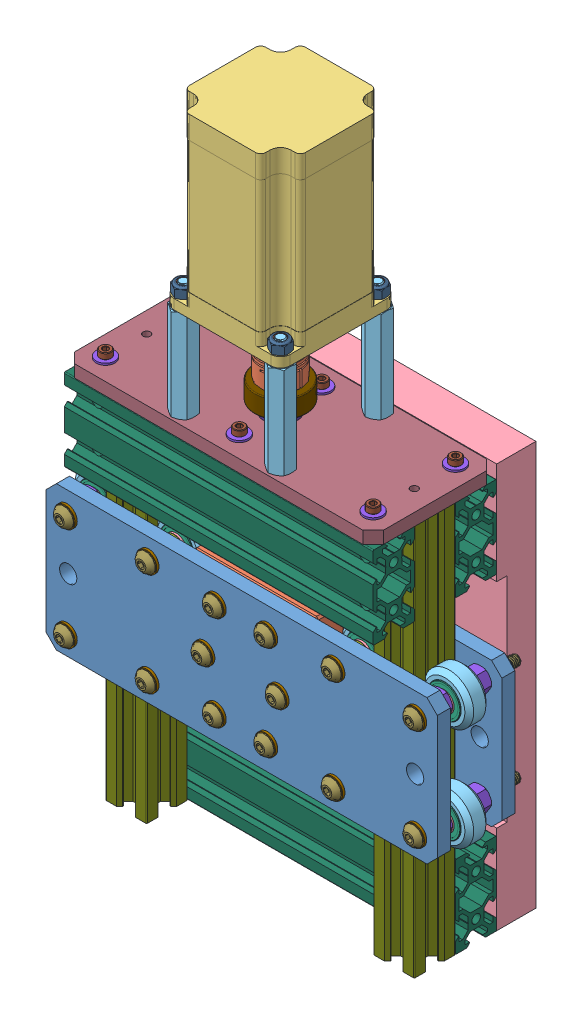
SolidWorks assembly Longitudinal Trim Assembly, configuration Default. Lengths in mm.
Overall size (193.6 327 79.96).
284 component instances, 29 part files, 72 mates.
Components (placement in the parent):
- Trim Sled Assembly-1: Trim Sled Assembly [Default] at origin size (193.6 74.69 53.02)
  - Trim Sled Plate-1: Trim Sled Plate [Default] at origin size (190 70 6.35)
  - Lead Screw Nut Clamshell-1: Lead Screw Nut Clamshell [Default] at origin size (60 70 12.5)
  - MISUMI Brass Lead Screw Flange Nut - MTSGR12-1: MISUMI Brass Lead Screw Flange Nut - MTSGR12 [Default] at (0 -15 30) x (0 1 0) z (0 0 1) size (30 44 24)
  - Lead Screw Nut Clamshell-2: Lead Screw Nut Clamshell [Default] at (0 0 60) x (-1 0 0) z (0 0 -1) size (60 70 12.5)
  - Inboard Wheel Stack-1: Inboard Wheel Stack [Default] at (-45.15 -25 23.5) size (23.9 23.9 25)
    - Xtreme Solid V Wheel Kit Assembly-1: Xtreme Solid V Wheel Kit Assembly [Default] at origin size (23.9 23.9 13)
      - Precision Shim - 10x5x1mm-1: Precision Shim - 10x5x1mm [Default] at origin size (10 10 1)
      - Xtreme Solid V Wheel Assembly-1: Xtreme Solid V Wheel Assembly [Default] at (45.15 25 -23.5) size (23.9 23.9 11)
        - Xtreme Solid V Wheel-1: Xtreme Solid V Wheel [Default] at (-45.15 -25 30) x (0 0 1) z (-1 0 0) size (10.2 23.9 23.9)
        - Wheel+Kit+-+5x16x5mm+Sealed+Radial+Ball+Bearing.step.f3d-1: Wheel+Kit+-+5x16x5mm+Sealed+Radial+Ball+Bearing.step.f3d [Default] at (-45.15 -25 30) x (0 1 0) z (-1 0 0) size (16 5 16)
        - Wheel+Kit+-+5x16x5mm+Sealed+Radial+Ball+Bearing.step.f3d-2: Wheel+Kit+-+5x16x5mm+Sealed+Radial+Ball+Bearing.step.f3d [Default] at (-45.15 -25 30) x (0 1 0) z (1 0 0) size (16 5 16)
      - Precision Shim - 10x5x1mm-2: Precision Shim - 10x5x1mm [Default] at (0 0 12) size (10 10 1)
    - Aluminum Spacer 6mm-1: Aluminum Spacer 6mm [Default] at (0 0 -6) size (10 10 6)
    - Aluminum Spacer 6mm-2: Aluminum Spacer 6mm [Default] at (0 0 13) size (10 10 6)
  - Inboard Wheel Stack_1-1: Inboard Wheel Stack_1 [Default] at (-45.15 25 23.5) size (23.9 23.9 25)
    - Xtreme Solid V Wheel Kit Assembly_1-1: Xtreme Solid V Wheel Kit Assembly_1 [Default] at origin size (23.9 23.9 13)
      - Precision Shim - 10x5x1mm-1: Precision Shim - 10x5x1mm [Default] at origin size (10 10 1)
      - Xtreme Solid V Wheel Assembly_1-1: Xtreme Solid V Wheel Assembly_1 [Default] at (45.15 55 -23.5) size (23.9 23.9 11)
        - Xtreme Solid V Wheel-1: Xtreme Solid V Wheel [Default] at (-45.15 -55 30) x (0 0 1) z (-1 0 0) size (10.2 23.9 23.9)
        - Wheel+Kit+-+5x16x5mm+Sealed+Radial+Ball+Bearing.step.f3d-1: Wheel+Kit+-+5x16x5mm+Sealed+Radial+Ball+Bearing.step.f3d [Default] at (-45.15 -55 30) x (0 1 0) z (-1 0 0) size (16 5 16)
        - Wheel+Kit+-+5x16x5mm+Sealed+Radial+Ball+Bearing.step.f3d-2: Wheel+Kit+-+5x16x5mm+Sealed+Radial+Ball+Bearing.step.f3d [Default] at (-45.15 -55 30) x (0 1 0) z (1 0 0) size (16 5 16)
      - Precision Shim - 10x5x1mm-2: Precision Shim - 10x5x1mm [Default] at (0 0 12) size (10 10 1)
    - Aluminum Spacer 6mm-1: Aluminum Spacer 6mm [Default] at (0 0 -6) size (10 10 6)
    - Aluminum Spacer 6mm-2: Aluminum Spacer 6mm [Default] at (0 0 13) size (10 10 6)
  - Inboard Wheel Stack_2-1: Inboard Wheel Stack_2 [Default] at (45.15 25 23.5) size (23.9 23.9 25)
    - Xtreme Solid V Wheel Kit Assembly_2-1: Xtreme Solid V Wheel Kit Assembly_2 [Default] at origin size (23.9 23.9 13)
      - Precision Shim - 10x5x1mm-1: Precision Shim - 10x5x1mm [Default] at origin size (10 10 1)
      - Xtreme Solid V Wheel Assembly_2-1: Xtreme Solid V Wheel Assembly_2 [Default] at (154.85 55 -23.5) size (23.9 23.9 11)
        - Xtreme Solid V Wheel-1: Xtreme Solid V Wheel [Default] at (-154.85 -55 30) x (0 0 1) z (-1 0 0) size (10.2 23.9 23.9)
        - Wheel+Kit+-+5x16x5mm+Sealed+Radial+Ball+Bearing.step.f3d-1: Wheel+Kit+-+5x16x5mm+Sealed+Radial+Ball+Bearing.step.f3d [Default] at (-154.85 -55 30) x (0 1 0) z (-1 0 0) size (16 5 16)
        - Wheel+Kit+-+5x16x5mm+Sealed+Radial+Ball+Bearing.step.f3d-2: Wheel+Kit+-+5x16x5mm+Sealed+Radial+Ball+Bearing.step.f3d [Default] at (-154.85 -55 30) x (0 1 0) z (1 0 0) size (16 5 16)
      - Precision Shim - 10x5x1mm-2: Precision Shim - 10x5x1mm [Default] at (0 0 12) size (10 10 1)
    - Aluminum Spacer 6mm-1: Aluminum Spacer 6mm [Default] at (0 0 -6) size (10 10 6)
    - Aluminum Spacer 6mm-2: Aluminum Spacer 6mm [Default] at (0 0 13) size (10 10 6)
  - Inboard Wheel Stack_3-1: Inboard Wheel Stack_3 [Default] at (45.15 -25 23.5) size (23.9 23.9 25)
    - Xtreme Solid V Wheel Kit Assembly_3-1: Xtreme Solid V Wheel Kit Assembly_3 [Default] at origin size (23.9 23.9 13)
      - Precision Shim - 10x5x1mm-1: Precision Shim - 10x5x1mm [Default] at origin size (10 10 1)
      - Xtreme Solid V Wheel Assembly_3-1: Xtreme Solid V Wheel Assembly_3 [Default] at (154.85 25 -23.5) size (23.9 23.9 11)
        - Xtreme Solid V Wheel-1: Xtreme Solid V Wheel [Default] at (-154.85 -25 30) x (0 0 1) z (-1 0 0) size (10.2 23.9 23.9)
        - Wheel+Kit+-+5x16x5mm+Sealed+Radial+Ball+Bearing.step.f3d-1: Wheel+Kit+-+5x16x5mm+Sealed+Radial+Ball+Bearing.step.f3d [Default] at (-154.85 -25 30) x (0 1 0) z (-1 0 0) size (16 5 16)
        - Wheel+Kit+-+5x16x5mm+Sealed+Radial+Ball+Bearing.step.f3d-2: Wheel+Kit+-+5x16x5mm+Sealed+Radial+Ball+Bearing.step.f3d [Default] at (-154.85 -25 30) x (0 1 0) z (1 0 0) size (16 5 16)
      - Precision Shim - 10x5x1mm-2: Precision Shim - 10x5x1mm [Default] at (0 0 12) size (10 10 1)
    - Aluminum Spacer 6mm-1: Aluminum Spacer 6mm [Default] at (0 0 -6) size (10 10 6)
    - Aluminum Spacer 6mm-2: Aluminum Spacer 6mm [Default] at (0 0 13) size (10 10 6)
  - Outboard Wheel Stack-1: Outboard Wheel Stack [Default] at (-84.85 -25.79 23.5) size (23.9 23.9 30)
    - Xtreme Solid V Wheel Kit Assembly_4-1: Xtreme Solid V Wheel Kit Assembly_4 [Default] at origin size (23.9 23.9 13)
      - Precision Shim - 10x5x1mm-1: Precision Shim - 10x5x1mm [Default] at origin size (10 10 1)
      - Xtreme Solid V Wheel Assembly_4-1: Xtreme Solid V Wheel Assembly_4 [Default] at (84.85 25.79 -23.5) size (23.9 23.9 11)
        - Xtreme Solid V Wheel-1: Xtreme Solid V Wheel [Default] at (-84.85 -25.79 30) x (0 0 1) z (-1 0 0) size (10.2 23.9 23.9)
        - Wheel+Kit+-+5x16x5mm+Sealed+Radial+Ball+Bearing.step.f3d-1: Wheel+Kit+-+5x16x5mm+Sealed+Radial+Ball+Bearing.step.f3d [Default] at (-84.85 -25.79 30) x (0 1 0) z (-1 0 0) size (16 5 16)
        - Wheel+Kit+-+5x16x5mm+Sealed+Radial+Ball+Bearing.step.f3d-2: Wheel+Kit+-+5x16x5mm+Sealed+Radial+Ball+Bearing.step.f3d [Default] at (-84.85 -25.79 30) x (0 1 0) z (1 0 0) size (16 5 16)
      - Precision Shim - 10x5x1mm-2: Precision Shim - 10x5x1mm [Default] at (0 0 12) size (10 10 1)
    - Eccentric Spacer 6mm-1: Eccentric Spacer 6mm [Default] at (0 0.79 -6) x (1 0 0) z (0 -1 0) size (11.55 8.5 10)
    - Eccentric Spacer 6mm-2: Eccentric Spacer 6mm [Default] at (0 0.79 19) x (-1 0 0) z (0 -1 0) size (11.55 8.5 10)
  - Outboard Wheel Stack_1-1: Outboard Wheel Stack_1 [Default] at (-84.85 24.21 23.5) size (23.9 23.9 30)
    - Xtreme Solid V Wheel Kit Assembly_5-1: Xtreme Solid V Wheel Kit Assembly_5 [Default] at origin size (23.9 23.9 13)
      - Precision Shim - 10x5x1mm-1: Precision Shim - 10x5x1mm [Default] at origin size (10 10 1)
      - Xtreme Solid V Wheel Assembly_5-1: Xtreme Solid V Wheel Assembly_5 [Default] at (84.85 55.79 -23.5) size (23.9 23.9 11)
        - Xtreme Solid V Wheel-1: Xtreme Solid V Wheel [Default] at (-84.85 -55.79 30) x (0 0 1) z (-1 0 0) size (10.2 23.9 23.9)
        - Wheel+Kit+-+5x16x5mm+Sealed+Radial+Ball+Bearing.step.f3d-1: Wheel+Kit+-+5x16x5mm+Sealed+Radial+Ball+Bearing.step.f3d [Default] at (-84.85 -55.79 30) x (0 1 0) z (-1 0 0) size (16 5 16)
        - Wheel+Kit+-+5x16x5mm+Sealed+Radial+Ball+Bearing.step.f3d-2: Wheel+Kit+-+5x16x5mm+Sealed+Radial+Ball+Bearing.step.f3d [Default] at (-84.85 -55.79 30) x (0 1 0) z (1 0 0) size (16 5 16)
      - Precision Shim - 10x5x1mm-2: Precision Shim - 10x5x1mm [Default] at (0 0 12) size (10 10 1)
    - Eccentric Spacer 6mm-1: Eccentric Spacer 6mm [Default] at (0 0.79 -6) x (1 0 0) z (0 -1 0) size (11.55 8.5 10)
    - Eccentric Spacer 6mm-2: Eccentric Spacer 6mm [Default] at (0 0.79 19) x (-1 0 0) z (0 -1 0) size (11.55 8.5 10)
  - Outboard Wheel Stack_2-1: Outboard Wheel Stack_2 [Default] at (84.85 24.21 23.5) size (23.9 23.9 30)
    - Xtreme Solid V Wheel Kit Assembly_6-1: Xtreme Solid V Wheel Kit Assembly_6 [Default] at origin size (23.9 23.9 13)
      - Precision Shim - 10x5x1mm-1: Precision Shim - 10x5x1mm [Default] at origin size (10 10 1)
      - Xtreme Solid V Wheel Assembly_6-1: Xtreme Solid V Wheel Assembly_6 [Default] at (115.15 55.79 -23.5) size (23.9 23.9 11)
        - Xtreme Solid V Wheel-1: Xtreme Solid V Wheel [Default] at (-115.15 -55.79 30) x (0 0 1) z (-1 0 0) size (10.2 23.9 23.9)
        - Wheel+Kit+-+5x16x5mm+Sealed+Radial+Ball+Bearing.step.f3d-1: Wheel+Kit+-+5x16x5mm+Sealed+Radial+Ball+Bearing.step.f3d [Default] at (-115.15 -55.79 30) x (0 1 0) z (-1 0 0) size (16 5 16)
        - Wheel+Kit+-+5x16x5mm+Sealed+Radial+Ball+Bearing.step.f3d-2: Wheel+Kit+-+5x16x5mm+Sealed+Radial+Ball+Bearing.step.f3d [Default] at (-115.15 -55.79 30) x (0 1 0) z (1 0 0) size (16 5 16)
      - Precision Shim - 10x5x1mm-2: Precision Shim - 10x5x1mm [Default] at (0 0 12) size (10 10 1)
    - Eccentric Spacer 6mm-1: Eccentric Spacer 6mm [Default] at (0 0.79 -6) x (1 0 0) z (0 -1 0) size (11.55 8.5 10)
    - Eccentric Spacer 6mm-2: Eccentric Spacer 6mm [Default] at (0 0.79 19) x (-1 0 0) z (0 -1 0) size (11.55 8.5 10)
  - Outboard Wheel Stack_3-1: Outboard Wheel Stack_3 [Default] at (84.85 -25.79 23.5) size (23.9 23.9 30)
    - Xtreme Solid V Wheel Kit Assembly_7-1: Xtreme Solid V Wheel Kit Assembly_7 [Default] at origin size (23.9 23.9 13)
      - Precision Shim - 10x5x1mm-1: Precision Shim - 10x5x1mm [Default] at origin size (10 10 1)
      - Xtreme Solid V Wheel Assembly_7-1: Xtreme Solid V Wheel Assembly_7 [Default] at (115.15 25.79 -23.5) size (23.9 23.9 11)
        - Xtreme Solid V Wheel-1: Xtreme Solid V Wheel [Default] at (-115.15 -25.79 30) x (0 0 1) z (-1 0 0) size (10.2 23.9 23.9)
        - Wheel+Kit+-+5x16x5mm+Sealed+Radial+Ball+Bearing.step.f3d-1: Wheel+Kit+-+5x16x5mm+Sealed+Radial+Ball+Bearing.step.f3d [Default] at (-115.15 -25.79 30) x (0 1 0) z (-1 0 0) size (16 5 16)
        - Wheel+Kit+-+5x16x5mm+Sealed+Radial+Ball+Bearing.step.f3d-2: Wheel+Kit+-+5x16x5mm+Sealed+Radial+Ball+Bearing.step.f3d [Default] at (-115.15 -25.79 30) x (0 1 0) z (1 0 0) size (16 5 16)
      - Precision Shim - 10x5x1mm-2: Precision Shim - 10x5x1mm [Default] at (0 0 12) size (10 10 1)
    - Eccentric Spacer 6mm-1: Eccentric Spacer 6mm [Default] at (0 0.79 -6) x (1 0 0) z (0 -1 0) size (11.55 8.5 10)
    - Eccentric Spacer 6mm-2: Eccentric Spacer 6mm [Default] at (0 0.79 19) x (-1 0 0) z (0 -1 0) size (11.55 8.5 10)
  - Trim Sled Plate-2: Trim Sled Plate [Default] at (0 0 31.35) size (190 70 6.35)
  - 93475A240-1: 93475A240 [Default] at (84.85 -25 48.85) x (0.893587 -0.448891 0) z (0 0 1) size (10 10 1.1)
  - 93475A240-2: 93475A240 [Default] at (84.85 -25 10.05) x (0.893587 -0.448891 0) z (0 0 1) size (10 10 1.1)
  - 93625A200 - M5 x 0.8 mm Nylon-Insert Locknut-1: 93625A200 - M5 x 0.8 mm Nylon-Insert Locknut [Default] at (84.85 -25 10.05) x (1 0 0) z (0 0 -1) size (8 9.24 5)
    - 93625A200 - M5 x 0.8 mm Nylon-Insert Locknut_2-1: 93625A200 - M5 x 0.8 mm Nylon-Insert Locknut_2 [Default] at origin size (8 9.24 5)
    - 93625A200 - M5 x 0.8 mm Nylon-Insert Locknut-1: 93625A200 - M5 x 0.8 mm Nylon-Insert Locknut [Default] at origin size (7.53 7.53 0.53)
  - 92095A228 - BHCS, M5-0.8 X 50, 18-8-1: 92095A228 - BHCS, M5-0.8 X 50, 18-8 [92095A228] at (84.85 -25 52.7) x (-0.790957 0.611872 0) z (0 0 1) size (9.5 9.5 53.02)
  - 93475A240-3: 93475A240 [Default] at (45.15 -25 48.85) x (0.953456 -0.301532 0) z (0 0 1) size (10 10 1.1)
  - 93475A240-4: 93475A240 [Default] at (45.15 -25 10.05) x (0.953456 -0.301532 0) z (0 0 1) size (10 10 1.1)
  - 93625A200 - M5 x 0.8 mm Nylon-Insert Locknut-2: 93625A200 - M5 x 0.8 mm Nylon-Insert Locknut [Default] at (45.15 -25 10.05) x (0.987351 0.158553 0) z (0 0 -1) size (8 9.24 5)
    - 93625A200 - M5 x 0.8 mm Nylon-Insert Locknut_2-1: 93625A200 - M5 x 0.8 mm Nylon-Insert Locknut_2 [Default] at origin size (8 9.24 5)
    - 93625A200 - M5 x 0.8 mm Nylon-Insert Locknut-1: 93625A200 - M5 x 0.8 mm Nylon-Insert Locknut [Default] at origin size (7.53 7.53 0.53)
  - 92095A228 - BHCS, M5-0.8 X 50, 18-8-2: 92095A228 - BHCS, M5-0.8 X 50, 18-8 [92095A228] at (45.15 -25 52.7) x (-0.877966 0.478723 0) z (0 0 1) size (9.5 9.5 53.02)
  - 93475A240-5: 93475A240 [Default] at (84.85 24.21 48.85) x (0.98409 -0.177672 0) z (0 0 1) size (10 10 1.1)
  - 93475A240-6: 93475A240 [Default] at (84.85 24.21 10.05) x (0.98409 -0.177672 0) z (0 0 1) size (10 10 1.1)
  - 93625A200 - M5 x 0.8 mm Nylon-Insert Locknut-3: 93625A200 - M5 x 0.8 mm Nylon-Insert Locknut [Default] at (84.85 24.21 10.05) x (0.959125 0.282984 0) z (0 0 -1) size (8 9.24 5)
    - 93625A200 - M5 x 0.8 mm Nylon-Insert Locknut_2-1: 93625A200 - M5 x 0.8 mm Nylon-Insert Locknut_2 [Default] at origin size (8 9.24 5)
    - 93625A200 - M5 x 0.8 mm Nylon-Insert Locknut-1: 93625A200 - M5 x 0.8 mm Nylon-Insert Locknut [Default] at origin size (7.53 7.53 0.53)
  - 92095A228 - BHCS, M5-0.8 X 50, 18-8-3: 92095A228 - BHCS, M5-0.8 X 50, 18-8 [92095A228] at (84.85 24.21 52.7) x (-0.931776 0.363033 0) z (0 0 1) size (9.5 9.5 53.02)
  - 93475A240-7: 93475A240 [Default] at (45.15 25 48.85) x (0.996366 -0.085169 0) z (0 0 1) size (10 10 1.1)
  - 93475A240-8: 93475A240 [Default] at (45.15 25 10.05) x (0.996366 -0.085169 0) z (0 0 1) size (10 10 1.1)
  - 93625A200 - M5 x 0.8 mm Nylon-Insert Locknut-4: 93625A200 - M5 x 0.8 mm Nylon-Insert Locknut [Default] at (45.15 25 10.05) x (0.928571 0.371154 0) z (0 0 -1) size (8 9.24 5)
    - 93625A200 - M5 x 0.8 mm Nylon-Insert Locknut_2-1: 93625A200 - M5 x 0.8 mm Nylon-Insert Locknut_2 [Default] at origin size (8 9.24 5)
    - 93625A200 - M5 x 0.8 mm Nylon-Insert Locknut-1: 93625A200 - M5 x 0.8 mm Nylon-Insert Locknut [Default] at origin size (7.53 7.53 0.53)
  - 92095A228 - BHCS, M5-0.8 X 50, 18-8-4: 92095A228 - BHCS, M5-0.8 X 50, 18-8 [92095A228] at (45.15 25 52.7) x (-0.961559 0.2746 0) z (0 0 1) size (9.5 9.5 53.02)
  - 93475A240-9: 93475A240 [Default] at (-45.15 -25 48.85) x (0.999525 -0.030802 0) z (0 0 1) size (10 10 1.1)
  - 93475A240-10: 93475A240 [Default] at (-45.15 -25 10.05) x (0.999525 -0.030802 0) z (0 0 1) size (10 10 1.1)
  - 93625A200 - M5 x 0.8 mm Nylon-Insert Locknut-5: 93625A200 - M5 x 0.8 mm Nylon-Insert Locknut [Default] at (-45.15 -25 10.05) x (0.906989 0.421154 0) z (0 0 -1) size (8 9.24 5)
    - 93625A200 - M5 x 0.8 mm Nylon-Insert Locknut_2-1: 93625A200 - M5 x 0.8 mm Nylon-Insert Locknut_2 [Default] at origin size (8 9.24 5)
    - 93625A200 - M5 x 0.8 mm Nylon-Insert Locknut-1: 93625A200 - M5 x 0.8 mm Nylon-Insert Locknut [Default] at origin size (7.53 7.53 0.53)
  - 92095A228 - BHCS, M5-0.8 X 50, 18-8-5: 92095A228 - BHCS, M5-0.8 X 50, 18-8 [92095A228] at (-45.15 -25 52.7) x (-0.975082 0.221847 0) z (0 0 1) size (9.5 9.5 53.02)
  - 93475A240-11: 93475A240 [Default] at (-84.85 -25.79 48.85) x (0.999778 -0.021077 0) z (0 0 1) size (10 10 1.1)
  - 93475A240-12: 93475A240 [Default] at (-84.85 -25.79 10.05) x (0.999778 -0.021077 0) z (0 0 1) size (10 10 1.1)
  - 93625A200 - M5 x 0.8 mm Nylon-Insert Locknut-6: 93625A200 - M5 x 0.8 mm Nylon-Insert Locknut [Default] at (-84.85 -25.79 10.05) x (0.902849 0.429957 0) z (0 0 -1) size (8 9.24 5)
    - 93625A200 - M5 x 0.8 mm Nylon-Insert Locknut_2-1: 93625A200 - M5 x 0.8 mm Nylon-Insert Locknut_2 [Default] at origin size (8 9.24 5)
    - 93625A200 - M5 x 0.8 mm Nylon-Insert Locknut-1: 93625A200 - M5 x 0.8 mm Nylon-Insert Locknut [Default] at origin size (7.53 7.53 0.53)
  - 92095A228 - BHCS, M5-0.8 X 50, 18-8-6: 92095A228 - BHCS, M5-0.8 X 50, 18-8 [92095A228] at (-84.85 -25.79 52.7) x (-0.977194 0.212351 0) z (0 0 1) size (9.5 9.5 53.02)
  - 93475A240-13: 93475A240 [Default] at (-45.15 25 48.85) x (0.998089 -0.061788 0) z (0 0 1) size (10 10 1.1)
  - 93475A240-14: 93475A240 [Default] at (-45.15 25 10.05) x (0.998089 -0.061788 0) z (0 0 1) size (10 10 1.1)
  - 93625A200 - M5 x 0.8 mm Nylon-Insert Locknut-7: 93625A200 - M5 x 0.8 mm Nylon-Insert Locknut [Default] at (-45.15 25 10.05) x (0.919615 0.39282 0) z (0 0 -1) size (8 9.24 5)
    - 93625A200 - M5 x 0.8 mm Nylon-Insert Locknut_2-1: 93625A200 - M5 x 0.8 mm Nylon-Insert Locknut_2 [Default] at origin size (8 9.24 5)
    - 93625A200 - M5 x 0.8 mm Nylon-Insert Locknut-1: 93625A200 - M5 x 0.8 mm Nylon-Insert Locknut [Default] at origin size (7.53 7.53 0.53)
  - 92095A228 - BHCS, M5-0.8 X 50, 18-8-7: 92095A228 - BHCS, M5-0.8 X 50, 18-8 [92095A228] at (-45.15 25 52.7) x (-0.967732 0.251983 0) z (0 0 1) size (9.5 9.5 53.02)
  - 93475A240-15: 93475A240 [Default] at (-84.85 24.21 48.85) x (0.987935 -0.154868 0) z (0 0 1) size (10 10 1.1)
  - 93475A240-16: 93475A240 [Default] at (-84.85 24.21 10.05) x (0.987935 -0.154868 0) z (0 0 1) size (10 10 1.1)
  - 93625A200 - M5 x 0.8 mm Nylon-Insert Locknut-8: 93625A200 - M5 x 0.8 mm Nylon-Insert Locknut [Default] at (-84.85 24.21 10.05) x (0.952324 0.305088 0) z (0 0 -1) size (8 9.24 5)
    - 93625A200 - M5 x 0.8 mm Nylon-Insert Locknut_2-1: 93625A200 - M5 x 0.8 mm Nylon-Insert Locknut_2 [Default] at origin size (8 9.24 5)
    - 93625A200 - M5 x 0.8 mm Nylon-Insert Locknut-1: 93625A200 - M5 x 0.8 mm Nylon-Insert Locknut [Default] at origin size (7.53 7.53 0.53)
  - 92095A228 - BHCS, M5-0.8 X 50, 18-8-8: 92095A228 - BHCS, M5-0.8 X 50, 18-8 [92095A228] at (-84.85 24.21 52.7) x (-0.939922 0.341389 0) z (0 0 1) size (9.5 9.5 53.02)
  - 93475A240-17: 93475A240 [Default] at (12.5 -23 48.85) x (0.597241 0.802062 0) z (0 0 1) size (10 10 1.1)
  - 93475A240-18: 93475A240 [Default] at (12.5 -23 10.05) x (0.597241 0.802062 0) z (0 0 1) size (10 10 1.1)
  - 93625A200 - M5 x 0.8 mm Nylon-Insert Locknut-9: 93625A200 - M5 x 0.8 mm Nylon-Insert Locknut [Default] at (12.5 -23 10.05) x (0.173648 0.984808 0) z (0 0 -1) size (8 9.24 5)
    - 93625A200 - M5 x 0.8 mm Nylon-Insert Locknut_2-1: 93625A200 - M5 x 0.8 mm Nylon-Insert Locknut_2 [Default] at origin size (8 9.24 5)
    - 93625A200 - M5 x 0.8 mm Nylon-Insert Locknut-1: 93625A200 - M5 x 0.8 mm Nylon-Insert Locknut [Default] at origin size (7.53 7.53 0.53)
  - 92095A228 - BHCS, M5-0.8 X 50, 18-8-9: 92095A228 - BHCS, M5-0.8 X 50, 18-8 [92095A228] at (12.5 -23 52.7) x (-0.739924 -0.67269 0) z (0 0 1) size (9.5 9.5 53.02)
  - 92095A228 - BHCS, M5-0.8 X 50, 18-8-10: 92095A228 - BHCS, M5-0.8 X 50, 18-8 [92095A228] at (-18 0 52.7) x (-0.739924 -0.67269 0) z (0 0 1) size (9.5 9.5 53.02)
  - 92095A228 - BHCS, M5-0.8 X 50, 18-8-11: 92095A228 - BHCS, M5-0.8 X 50, 18-8 [92095A228] at (-12.5 -23 52.7) x (-0.739924 -0.67269 0) z (0 0 1) size (9.5 9.5 53.02)
  - 92095A228 - BHCS, M5-0.8 X 50, 18-8-12: 92095A228 - BHCS, M5-0.8 X 50, 18-8 [92095A228] at (-12.5 23 52.7) x (-0.739924 -0.67269 0) z (0 0 1) size (9.5 9.5 53.02)
  - 92095A228 - BHCS, M5-0.8 X 50, 18-8-13: 92095A228 - BHCS, M5-0.8 X 50, 18-8 [92095A228] at (18 0 52.7) x (-0.739924 -0.67269 0) z (0 0 1) size (9.5 9.5 53.02)
  - 92095A228 - BHCS, M5-0.8 X 50, 18-8-14: 92095A228 - BHCS, M5-0.8 X 50, 18-8 [92095A228] at (12.5 23 52.7) x (-0.739924 -0.67269 0) z (0 0 1) size (9.5 9.5 53.02)
  - 93625A200 - M5 x 0.8 mm Nylon-Insert Locknut-10: 93625A200 - M5 x 0.8 mm Nylon-Insert Locknut [Default] at (-18 0 10.05) x (0.173648 0.984808 0) z (0 0 -1) size (8 9.24 5)
    - 93625A200 - M5 x 0.8 mm Nylon-Insert Locknut_2-1: 93625A200 - M5 x 0.8 mm Nylon-Insert Locknut_2 [Default] at origin size (8 9.24 5)
    - 93625A200 - M5 x 0.8 mm Nylon-Insert Locknut-1: 93625A200 - M5 x 0.8 mm Nylon-Insert Locknut [Default] at origin size (7.53 7.53 0.53)
  - 93625A200 - M5 x 0.8 mm Nylon-Insert Locknut-11: 93625A200 - M5 x 0.8 mm Nylon-Insert Locknut [Default] at (-12.5 -23 10.05) x (0.173648 0.984808 0) z (0 0 -1) size (8 9.24 5)
    - 93625A200 - M5 x 0.8 mm Nylon-Insert Locknut_2-1: 93625A200 - M5 x 0.8 mm Nylon-Insert Locknut_2 [Default] at origin size (8 9.24 5)
    - 93625A200 - M5 x 0.8 mm Nylon-Insert Locknut-1: 93625A200 - M5 x 0.8 mm Nylon-Insert Locknut [Default] at origin size (7.53 7.53 0.53)
  - 93625A200 - M5 x 0.8 mm Nylon-Insert Locknut-12: 93625A200 - M5 x 0.8 mm Nylon-Insert Locknut [Default] at (-12.5 23 10.05) x (0.173648 0.984808 0) z (0 0 -1) size (8 9.24 5)
    - 93625A200 - M5 x 0.8 mm Nylon-Insert Locknut_2-1: 93625A200 - M5 x 0.8 mm Nylon-Insert Locknut_2 [Default] at origin size (8 9.24 5)
    - 93625A200 - M5 x 0.8 mm Nylon-Insert Locknut-1: 93625A200 - M5 x 0.8 mm Nylon-Insert Locknut [Default] at origin size (7.53 7.53 0.53)
  - 93625A200 - M5 x 0.8 mm Nylon-Insert Locknut-13: 93625A200 - M5 x 0.8 mm Nylon-Insert Locknut [Default] at (18 0 10.05) x (0.173648 0.984808 0) z (0 0 -1) size (8 9.24 5)
    - 93625A200 - M5 x 0.8 mm Nylon-Insert Locknut_2-1: 93625A200 - M5 x 0.8 mm Nylon-Insert Locknut_2 [Default] at origin size (8 9.24 5)
    - 93625A200 - M5 x 0.8 mm Nylon-Insert Locknut-1: 93625A200 - M5 x 0.8 mm Nylon-Insert Locknut [Default] at origin size (7.53 7.53 0.53)
  - 93625A200 - M5 x 0.8 mm Nylon-Insert Locknut-14: 93625A200 - M5 x 0.8 mm Nylon-Insert Locknut [Default] at (12.5 23 10.05) x (0.173648 0.984808 0) z (0 0 -1) size (8 9.24 5)
    - 93625A200 - M5 x 0.8 mm Nylon-Insert Locknut_2-1: 93625A200 - M5 x 0.8 mm Nylon-Insert Locknut_2 [Default] at origin size (8 9.24 5)
    - 93625A200 - M5 x 0.8 mm Nylon-Insert Locknut-1: 93625A200 - M5 x 0.8 mm Nylon-Insert Locknut [Default] at origin size (7.53 7.53 0.53)
  - 93475A240-19: 93475A240 [Default] at (-18 0 10.05) x (0.597241 0.802062 0) z (0 0 1) size (10 10 1.1)
  - 93475A240-20: 93475A240 [Default] at (-12.5 -23 10.05) x (0.597241 0.802062 0) z (0 0 1) size (10 10 1.1)
  - 93475A240-21: 93475A240 [Default] at (-12.5 23 10.05) x (0.597241 0.802062 0) z (0 0 1) size (10 10 1.1)
  - 93475A240-22: 93475A240 [Default] at (18 0 10.05) x (0.597241 0.802062 0) z (0 0 1) size (10 10 1.1)
  - 93475A240-23: 93475A240 [Default] at (12.5 23 10.05) x (0.597241 0.802062 0) z (0 0 1) size (10 10 1.1)
  - 93475A240-24: 93475A240 [Default] at (-18 0 48.85) x (0.597241 0.802062 0) z (0 0 1) size (10 10 1.1)
  - 93475A240-25: 93475A240 [Default] at (-12.5 -23 48.85) x (0.597241 0.802062 0) z (0 0 1) size (10 10 1.1)
  - 93475A240-26: 93475A240 [Default] at (-12.5 23 48.85) x (0.597241 0.802062 0) z (0 0 1) size (10 10 1.1)
  - 93475A240-27: 93475A240 [Default] at (18 0 48.85) x (0.597241 0.802062 0) z (0 0 1) size (10 10 1.1)
  - 93475A240-28: 93475A240 [Default] at (12.5 23 48.85) x (0.597241 0.802062 0) z (0 0 1) size (10 10 1.1)
- Rear Plate Assembly-1: Rear Plate Assembly [Default] at origin size (150 6 60)
  - Rear Plate-1: Rear Plate [Default] at origin size (150 6 60)
  - 6658K734-1: 6658K734 [Default] at (0 98 30) x (1 0 0) z (0 -1 0) size (12.03 12.03 6)
- Aft Frame Assembly-1: Aft Frame Assembly [Default] at origin size (150 190 60)
  - V-Slot 20x40x150 Linear Rail-1: V-Slot 20x40x150 Linear Rail [Default] at (-75 75 10) x (0 0 -1) z (1 0 0) size (20 40 150)
  - V-Slot 20x20x190 Linear Rail Tapped Ends-1: V-Slot 20x20x190 Linear Rail Tapped Ends [Default] at (65 95 30) x (1 0 0) z (0 -1 0) size (20 20 190)
  - V-Slot 20x20x190 Linear Rail Tapped Ends-2: V-Slot 20x20x190 Linear Rail Tapped Ends [Default] at (-65 95 30) x (1 0 0) z (0 -1 0) size (20 20 190)
  - V-Slot 20x40x150 Linear Rail-2: V-Slot 20x40x150 Linear Rail [Default] at (-75 75 50) x (0 0 -1) z (1 0 0) size (20 40 150)
- V-Slot 20x40x150 Linear Rail-1: V-Slot 20x40x150 Linear Rail [Default] at (-75 -75 10) x (0 0 -1) z (1 0 0) size (20 40 150)
- 7806K630-1: 7806K630 [Default] at (0 92.5 30) size (16 5.01 16)
- 7806K630-2: 7806K630 [Default] at (0 103.5 30) size (16 5.01 16)
- 57445K24 - 8mm Clamping Shaft Collar-1: 57445K24 - 8mm Clamping Shaft Collar [Default] at (0 110.5 30) x (1 0 0) z (0 1 0) size (25 25.02 9.05)
- MTSBRA12-160-S35-Q8-1: MTSBRA12-160-S35-Q8 [Default] at (0 125 30) x (1 0 0) z (0 -1 0) size (11.91 11.91 160)
- 819368020915 - Flexible Coupling 5mm x 0.25in-1: 819368020915 - Flexible Coupling 5mm x 0.25in [Default] at (0 115.4 30) x (1 0 0) z (0 -1 0) size (20 20 25)
- 819368021257 - Nema 23 High Torque Stepper Motor-1: 819368021257 - Nema 23 High Torque Stepper Motor [Default] at (0 146 30) x (1 0 0) z (0 -1 0) size (56.4 56.4 106.6)
- Trim Riser Board-1: Trim Riser Board [Default] at origin size (150 196.35 19.05)
- 93655A248 - STANDOFF, MALE-TO-FEMALE, M5-0.8 X 12.7 THD DPTH X 10 HEX X 45L, 18-8-1: 93655A248 - STANDOFF, MALE-TO-FEMALE, M5-0.8 X 12.7 THD DPTH X 10 HEX X 45L, 18-8 [93655A248] at (23.57 128.5 53.57) x (0 1 0) z (-0.546944 0 0.837169) size (55.57 11.55 10)
- 93625A200 - M5 x 0.8 mm Nylon-Insert Locknut-9: 93625A200 - M5 x 0.8 mm Nylon-Insert Locknut [Default] at (23.57 150.8 53.57) x (0.549411 0 0.835552) z (0 1 0) size (8 9.24 5)
  - 93625A200 - M5 x 0.8 mm Nylon-Insert Locknut_2-1: 93625A200 - M5 x 0.8 mm Nylon-Insert Locknut_2 [Default] at origin size (8 9.24 5)
  - 93625A200 - M5 x 0.8 mm Nylon-Insert Locknut-1: 93625A200 - M5 x 0.8 mm Nylon-Insert Locknut [Default] at origin size (7.53 7.53 0.53)
- 92125A107 - FHS, 90 DEG, M5-0.8 X 15, 18-8-1: 92125A107 - FHS, 90 DEG, M5-0.8 X 15, 18-8 [92125A107] at (23.57 95.9 53.57) x (-0.028612 0 -0.999591) z (0 -1 0) size (10 10 15.47)
- 92125A107 - FHS, 90 DEG, M5-0.8 X 15, 18-8-2: 92125A107 - FHS, 90 DEG, M5-0.8 X 15, 18-8 [92125A107] at (23.57 95.9 6.43) x (-0.028612 0 -0.999591) z (0 -1 0) size (10 10 15.47)
- 92125A107 - FHS, 90 DEG, M5-0.8 X 15, 18-8-3: 92125A107 - FHS, 90 DEG, M5-0.8 X 15, 18-8 [92125A107] at (-23.57 95.9 6.43) x (-0.028612 0 -0.999591) z (0 -1 0) size (10 10 15.47)
- 92125A107 - FHS, 90 DEG, M5-0.8 X 15, 18-8-4: 92125A107 - FHS, 90 DEG, M5-0.8 X 15, 18-8 [92125A107] at (-23.57 95.9 53.57) x (-0.028612 0 -0.999591) z (0 -1 0) size (10 10 15.47)
- 93625A200 - M5 x 0.8 mm Nylon-Insert Locknut-10: 93625A200 - M5 x 0.8 mm Nylon-Insert Locknut [Default] at (23.57 150.8 6.43) x (0.549411 0 0.835552) z (0 1 0) size (8 9.24 5)
  - 93625A200 - M5 x 0.8 mm Nylon-Insert Locknut_2-1: 93625A200 - M5 x 0.8 mm Nylon-Insert Locknut_2 [Default] at origin size (8 9.24 5)
  - 93625A200 - M5 x 0.8 mm Nylon-Insert Locknut-1: 93625A200 - M5 x 0.8 mm Nylon-Insert Locknut [Default] at origin size (7.53 7.53 0.53)
- 93625A200 - M5 x 0.8 mm Nylon-Insert Locknut-11: 93625A200 - M5 x 0.8 mm Nylon-Insert Locknut [Default] at (-23.57 150.8 6.43) x (0.549411 0 0.835552) z (0 1 0) size (8 9.24 5)
  - 93625A200 - M5 x 0.8 mm Nylon-Insert Locknut_2-1: 93625A200 - M5 x 0.8 mm Nylon-Insert Locknut_2 [Default] at origin size (8 9.24 5)
  - 93625A200 - M5 x 0.8 mm Nylon-Insert Locknut-1: 93625A200 - M5 x 0.8 mm Nylon-Insert Locknut [Default] at origin size (7.53 7.53 0.53)
- 93625A200 - M5 x 0.8 mm Nylon-Insert Locknut-12: 93625A200 - M5 x 0.8 mm Nylon-Insert Locknut [Default] at (-23.57 150.8 53.57) x (0.549411 0 0.835552) z (0 1 0) size (8 9.24 5)
  - 93625A200 - M5 x 0.8 mm Nylon-Insert Locknut_2-1: 93625A200 - M5 x 0.8 mm Nylon-Insert Locknut_2 [Default] at origin size (8 9.24 5)
  - 93625A200 - M5 x 0.8 mm Nylon-Insert Locknut-1: 93625A200 - M5 x 0.8 mm Nylon-Insert Locknut [Default] at origin size (7.53 7.53 0.53)
- 93655A248 - STANDOFF, MALE-TO-FEMALE, M5-0.8 X 12.7 THD DPTH X 10 HEX X 45L, 18-8-2: 93655A248 - STANDOFF, MALE-TO-FEMALE, M5-0.8 X 12.7 THD DPTH X 10 HEX X 45L, 18-8 [93655A248] at (23.57 128.5 6.43) x (0 1 0) z (-0.546944 0 0.837169) size (55.57 11.55 10)
- 93655A248 - STANDOFF, MALE-TO-FEMALE, M5-0.8 X 12.7 THD DPTH X 10 HEX X 45L, 18-8-3: 93655A248 - STANDOFF, MALE-TO-FEMALE, M5-0.8 X 12.7 THD DPTH X 10 HEX X 45L, 18-8 [93655A248] at (-23.57 128.5 6.43) x (0 1 0) z (-0.546944 0 0.837169) size (55.57 11.55 10)
- 93655A248 - STANDOFF, MALE-TO-FEMALE, M5-0.8 X 12.7 THD DPTH X 10 HEX X 45L, 18-8-4: 93655A248 - STANDOFF, MALE-TO-FEMALE, M5-0.8 X 12.7 THD DPTH X 10 HEX X 45L, 18-8 [93655A248] at (-23.57 128.5 53.57) x (0 1 0) z (-0.546944 0 0.837169) size (55.57 11.55 10)
- HNTTBS5-3 - NUT, PRE-INSERTION, M3 X 10 SQ, 18-8-1: HNTTBS5-3 - NUT, PRE-INSERTION, M3 X 10 SQ, 18-8 [Default] at (65 -85 21.8) x (0 0 -1) z (0 -1 0) size (2.7 10 10)
- 91100A120 - WASHER, M3 X 9 OD, 18-8-1: 91100A120 - WASHER, M3 X 9 OD, 18-8 [93475A210] at (65 -85 17.3) x (0.993328 0.115328 0) z (0 0 1) size (9 9 0.9)
- 94500A222 - BHCS, M3-0.5 X 8, 316 SS-1: 94500A222 - BHCS, M3-0.5 X 8, 316 SS [94500A222] at (65 -85 15.65) x (-0.923728 -0.383049 0) z (0 0 -1) size (5.7 5.7 9.95)
- HNTTBS5-3 - NUT, PRE-INSERTION, M3 X 10 SQ, 18-8-2: HNTTBS5-3 - NUT, PRE-INSERTION, M3 X 10 SQ, 18-8 [Default] at (65 -65 21.8) x (0 0 -1) z (0 -1 0) size (2.7 10 10)
